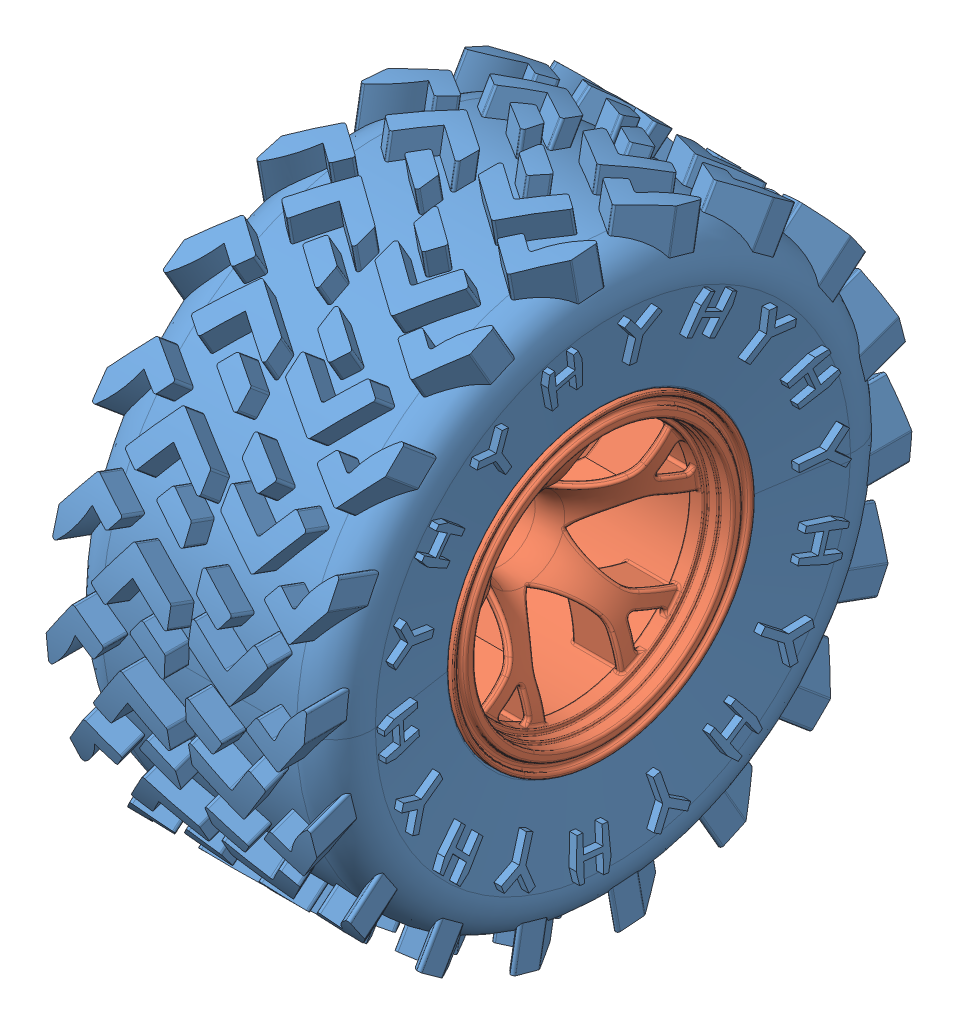
SolidWorks assembly Plastic Wheel 130mm, configuration Default. Lengths in mm.
Overall size (57.88 126.13 125.05).
3 component instances, 2 part files, 0 mates.
Components (placement in the parent):
- Plastic Wheel 130mm.STEP-1: Plastic Wheel 130mm.STEP [Default] at origin size (57.88 126.13 125.05)
  - Tyre.STEP-1: Tyre.STEP [Default] at origin size (57.88 126.13 125.05)
  - Plastic Rim.STEP-1: Plastic Rim.STEP [Default] at (-24.3 0 0) x (0 -0.536317 -0.844017) z (0 -0.844017 0.536317) size (62 50 62)
